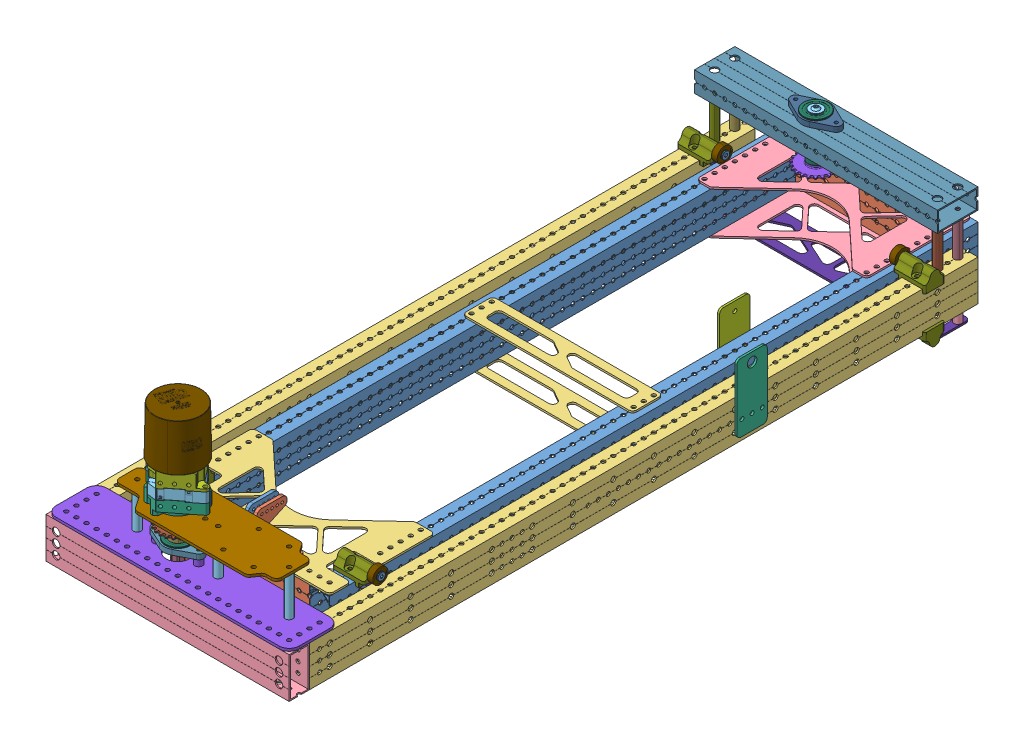
SolidWorks assembly Elevator Assembly 3.0, configuration Default. Lengths in mm.
Overall size (311.03 238.34 907.36).
103 component instances, 46 part files, 163 mates.
Components (placement in the parent):
- 32inTubeStock-1: 32inTubeStock [Default] at (147.012 423.1257 1446.8134) size (25.4 50.8 812.8)
- 32inTubeStock-2: 32inTubeStock [Default] at (-56.188 423.1257 1446.8134) size (25.4 50.8 812.8)
- 7inRevTube-1: 7inRevTube [Default] at (1137.612 423.1257 1065.8134) x (0 0 -1) z (1 0 0) size (25.4 50.8 177.8)
- 7inRevTube-2: 7inRevTube [Default] at (1137.612 423.1257 278.4134) x (0 0 -1) z (1 0 0) size (25.4 50.8 177.8)
- WCP-EX-0018-005(2)^Assem1-1: WCP-EX-0018-005(2)^Assem1 [Default] at (185.112 423.1257 519.7134) x (0 0 1) z (-1 0 0) size (838.2 50.8 25.4)
- WCP-EX-0018-001(2)^Assem1-1: WCP-EX-0018-001(2)^Assem1 [Default] at (45.412 423.1257 1154.7134) size (304.8 50.8 25.4)
- WCP-EX-0018-005(2)^Assem1-2: WCP-EX-0018-005(2)^Assem1 [Default] at (-94.288 423.1257 519.7134) x (0 0 1) z (-1 0 0) size (838.2 50.8 25.4)
- REV-21-2102-4-1-cartridge-1: REV-21-2102-4-1-cartridge [Default] at (20.0926 531.0257 1129.1434) x (0.78617 0 -0.61801) z (0 -1 0) size (61.91 50.8 16.85)
- REV-21-2104-hex-socket-output-1: REV-21-2104-hex-socket-output [Default] at (20.0961 515.2007 1129.1406) x (0 -1 0) z (-0.78617 0 0.61801) size (23.2 50.8 61.92)
- REV-21-2106-universal-input-1: REV-21-2106-universal-input [Default] at (20.0926 546.8507 1129.1434) x (0.78617 0 -0.61801) z (0 -1 0) size (61.91 50.8 19.05)
- Copy (3) of Copy of WCP-0308 Rev1^Elevator Assembly 3.0-3: Copy (3) of Copy of WCP-0308 Rev1^Elevator Assembly 3.0 [Default] at (45.4854 454.8757 1128.4014) x (0 1 0) z (-0.838797 0 -0.544444) size (8.64 9.5 9.6) (virtual)
- Motor_Mounting_Plate-1: Motor_Mounting_Plate [Default] at (-30.7773 505.6757 1129.3134) x (1 0 0) z (0 0 -1) size (209.55 3.17 69.85)
- Copy of Copy of WCP-0800_500_hex_collar_high_strength^Elevator Assembly 3.0-1: Copy of Copy of WCP-0800_500_hex_collar_high_strength^Elevator Assembly 3.0 [Default] at (20.0961 492.0867 1129.1406) x (0.837169 0 0.546944) z (0 1 0) size (28.56 28.57 9.53) (virtual)
- Copy of Copy of WCP-0560 Rev1^Elevator Assembly 3.0-1: Copy of Copy of WCP-0560 Rev1^Elevator Assembly 3.0 [Default] at (20.0961 482.5617 1129.1406) x (0.312597 0 0.949886) z (0 -1 0) size (47.96 47.68 9.53) (virtual)
- Copy of Copy of WCP-0789_250L_500_hex^Elevator Assembly 3.0-1: Copy of Copy of WCP-0789_250L_500_hex^Elevator Assembly 3.0 [Default] at (20.0961 471.4492 1129.1406) x (-0.74566 0 -0.666327) z (0 1 0) size (19.5 19.5 6.35) (virtual)
- 1_2ThunderHex-1: 1_2ThunderHex [Default] at (20.0961 872.3882 1129.1406) x (0.204226 0 -0.978924) z (0 1 0) size (13.74 12.75 101.6)
- Copy of Copy of WCP-0476 Rev1^Elevator Assembly 3.0-1: Copy of Copy of WCP-0476 Rev1^Elevator Assembly 3.0 [Default] at (20.0961 463.5117 1129.1406) x (-0.999576 0 0.029102) z (0 -1 0) size (63.5 34.92 6.35) (virtual)
- WCP-0785_0_500_flanged_thunderhex_bearing.step-3: WCP-0785_0_500_flanged_thunderhex_bearing.step [Default] at (20.0961 464.3055 1129.1406) x (0.837169 0 0.546944) z (0 1 0) size (31.12 31.12 7.94)
- Copy (3) of Copy of WCP-0308 Rev1^Elevator Assembly 3.0-4: Copy (3) of Copy of WCP-0308 Rev1^Elevator Assembly 3.0 [Default] at (-5.2931 454.8757 1129.8798) x (0 1 0) z (0.450792 0 -0.892629) size (8.64 9.5 9.6) (virtual)
- Copy of WCP-0323 - Elevator Clamping Block-1-1: Copy of WCP-0323 - Elevator Clamping Block-1 [Default] at (159.7755 448.5257 1034.0634) x (0 -1 0) z (1 0 0) size (29.22 25.41 49.35)
  - WCP-0323-001 Rev2^Copy of WCP-0323 - Elevator Clamping Block-1-1: WCP-0323-001 Rev2^Copy of WCP-0323 - Elevator Clamping Block-1 [Default] at origin size (20.38 25.41 40.49) (virtual)
  - WCP-0498 Rev1^Copy of WCP-0323 - Elevator Clamping Block-1-1: WCP-0498 Rev1^Copy of WCP-0323 - Elevator Clamping Block-1 [Default] at (2.254 0 6.7) x (0 0.307359 0.951594) z (-1 0 0) size (12 12 4) (virtual)
  - WCP-0212_0_250_radial_bearing^Copy of WCP-0323 - Elevator Clamping Block-1-1: WCP-0212_0_250_radial_bearing^Copy of WCP-0323 - Elevator Clamping Block-1 [Default] at (-9.525 0 15.4781) size (19.05 19.05 7.14) (virtual)
  - WCP-0473 Rev1^Copy of WCP-0323 - Elevator Clamping Block-1-1: WCP-0473 Rev1^Copy of WCP-0323 - Elevator Clamping Block-1 [Default] at (-9.525 0 10.4394) x (-0.082744 -0.996571 0) z (-0.996571 0.082744 0) size (9.53 20.65 9.53) (virtual)
  - #8-32 x .25L BHCS^Copy of WCP-0323 - Elevator Clamping Block-1-1: #8-32 x .25L BHCS^Copy of WCP-0323 - Elevator Clamping Block-1 [Default] at (6.7178 0 6.7) x (0 -0.337236 -0.94142) z (1 0 0) size (10.28 8 12.02) (virtual)
- Inside_Bottom_Plate-1: Inside_Bottom_Plate [Default] at (-738.7858 448.5257 1008.0258) x (0 0 1) z (0 1 0) size (132.08 228.6 2.29)
- Copy of WCP-0323 - Elevator Clamping Block-1-2: Copy of WCP-0323 - Elevator Clamping Block-1 [Default] at (172.3485 448.5257 360.9634) x (0 -1 0) z (-1 0 0) size (29.22 25.41 49.35)
  - WCP-0323-001 Rev2^Copy of WCP-0323 - Elevator Clamping Block-1-1: WCP-0323-001 Rev2^Copy of WCP-0323 - Elevator Clamping Block-1 [Default] at origin size (20.38 25.41 40.49) (virtual)
  - WCP-0498 Rev1^Copy of WCP-0323 - Elevator Clamping Block-1-1: WCP-0498 Rev1^Copy of WCP-0323 - Elevator Clamping Block-1 [Default] at (2.254 0 6.7) x (0 0.307359 0.951594) z (-1 0 0) size (12 12 4) (virtual)
  - WCP-0212_0_250_radial_bearing^Copy of WCP-0323 - Elevator Clamping Block-1-1: WCP-0212_0_250_radial_bearing^Copy of WCP-0323 - Elevator Clamping Block-1 [Default] at (-9.525 0 15.4781) size (19.05 19.05 7.14) (virtual)
  - WCP-0473 Rev1^Copy of WCP-0323 - Elevator Clamping Block-1-1: WCP-0473 Rev1^Copy of WCP-0323 - Elevator Clamping Block-1 [Default] at (-9.525 0 10.4394) x (-0.082744 -0.996571 0) z (-0.996571 0.082744 0) size (9.53 20.65 9.53) (virtual)
  - #8-32 x .25L BHCS^Copy of WCP-0323 - Elevator Clamping Block-1-1: #8-32 x .25L BHCS^Copy of WCP-0323 - Elevator Clamping Block-1 [Default] at (6.7178 0 6.7) x (0 -0.337236 -0.94142) z (1 0 0) size (10.28 8 12.02) (virtual)
- Inside_Top_Plate-1: Inside_Top_Plate [Default] at (712.3991 448.5257 509.6002) x (0 0 -1) z (0 1 0) size (132.08 213.36 2.29)
- Copy of Copy of WCP-0571 Rev1^Elevator Assembly 3.0-1: Copy of Copy of WCP-0571 Rev1^Elevator Assembly 3.0 [Default] at (20.012 535.6604 329.2134) x (-0.49457 0 -0.869138) z (0 1 0) size (15.88 15.88 15.71) (virtual)
- Copy (2) of Copy of WCP-0571 Rev1^Elevator Assembly 3.0-2: Copy (2) of Copy of WCP-0571 Rev1^Elevator Assembly 3.0 [Default] at (20.012 466.166 329.2134) x (-0.946289 0 0.323321) z (0 -1 0) size (15.88 15.88 15.71) (virtual)
- Copy of Copy of WCP-0599 Rev1^Elevator Assembly 3.0-1: Copy of Copy of WCP-0599 Rev1^Elevator Assembly 3.0 [Default] at (20.012 500.9132 329.2134) x (0 -1 0) z (-0.783433 0 0.621476) size (63.5 12.67 13.72) (virtual)
- Copy of Copy (2) of WCP-0560 Rev1^Elevator Assembly 3.0-1: Copy of Copy (2) of WCP-0560 Rev1^Elevator Assembly 3.0 [Default] at (20.012 473.9257 329.2134) x (0.367735 0 -0.929931) z (0 -1 0) size (47.96 47.68 9.53) (virtual)
- WCP-0785_0_500_flanged_thunderhex_bearing.step-4: WCP-0785_0_500_flanged_thunderhex_bearing.step [Default] at (20.012 495.357 329.2134) x (-0.189996 0 -0.981785) z (0 -1 0) size (31.12 31.12 7.94)
- Copy (2) of Copy of WCP-0476 Rev1^Elevator Assembly 3.0-2: Copy (2) of Copy of WCP-0476 Rev1^Elevator Assembly 3.0 [Default] at (20.012 496.1507 329.2134) x (1 0 0) z (0 1 0) size (63.5 34.92 6.35) (virtual)
- WCP-0785_0_500_flanged_thunderhex_bearing.step-5: WCP-0785_0_500_flanged_thunderhex_bearing.step [Default] at (20.012 528.6945 329.2134) x (0.679938 0 -0.73327) z (0 1 0) size (31.12 31.12 7.94)
- Copy (3) of Copy of WCP-0476 Rev1^Elevator Assembly 3.0-3: Copy (3) of Copy of WCP-0476 Rev1^Elevator Assembly 3.0 [Default] at (20.012 527.9007 329.2134) x (1 0 0) z (0 -1 0) size (63.5 34.92 6.35) (virtual)
- Copy of Copy of WCP-0207 Rev1^Elevator Assembly 3.0-1: Copy of Copy of WCP-0207 Rev1^Elevator Assembly 3.0 [Default] at (185.112 473.9257 341.9134) x (0 -1 0) z (-0.448341 0 -0.893863) size (50.8 9.5 9.5) (virtual)
- Copy (2) of Copy of WCP-0207 Rev1^Elevator Assembly 3.0-2: Copy (2) of Copy of WCP-0207 Rev1^Elevator Assembly 3.0 [Default] at (-94.288 473.9257 316.5134) x (0 -1 0) z (-0.997465 0 0.071155) size (50.8 9.5 9.5) (virtual)
- Copy (3) of Copy of WCP-0207 Rev1^Elevator Assembly 3.0-3: Copy (3) of Copy of WCP-0207 Rev1^Elevator Assembly 3.0 [Default] at (185.112 473.9257 316.5134) x (0 -1 0) z (0.909972 0 0.414669) size (50.8 9.5 9.5) (virtual)
- WCP-EX-0018-002(2)^Elevator Assembly Updated 2.0-2: WCP-EX-0018-002(2)^Elevator Assembly Updated 2.0 [Default] at (45.412 512.0257 329.2134) x (1 0 0) z (0 -1 0) size (304.8 50.8 25.4)
- WCP-0790_500L_500_hex.step-1: WCP-0790_500L_500_hex.step [Default] at (20.012 485.0382 329.2134) x (0.992611 0 -0.121342) z (0 -1 0) size (19.5 19.5 12.7)
- Copy (4) of Copy of WCP-0207 Rev1^Elevator Assembly 3.0-4: Copy (4) of Copy of WCP-0207 Rev1^Elevator Assembly 3.0 [Default] at (-94.288 473.9257 341.9134) x (0 -1 0) z (0.710119 0 0.704082) size (50.8 9.5 9.5) (virtual)
- Outside_Top_Plate-1: Outside_Top_Plate [Default] at (185.112 378.6757 316.5134) x (0 0 1) z (0 -1 0) size (45.72 289.24 2.29)
- Part4^Elevator Assembly 3.0-1: Part4^Elevator Assembly 3.0 [Default] at origin (virtual)
- Neo1.1_REV-21-1650-V1.1-1: Neo1.1_REV-21-1650-V1.1 [Default] at (20.0926 556.3757 1129.1434) x (0.451737 0 0.892151) z (0 -1 0) size (68.13 68.01 93.35)
- Copy of WCP-0323 - Elevator Clamping Block-1-9: Copy of WCP-0323 - Elevator Clamping Block-1 [Default] at (-68.9515 448.5257 1034.0634) x (0 -1 0) z (-1 0 0) size (29.22 25.41 49.35)
  - WCP-0323-001 Rev2^Copy of WCP-0323 - Elevator Clamping Block-1-1: WCP-0323-001 Rev2^Copy of WCP-0323 - Elevator Clamping Block-1 [Default] at origin size (20.38 25.41 40.49) (virtual)
  - WCP-0498 Rev1^Copy of WCP-0323 - Elevator Clamping Block-1-1: WCP-0498 Rev1^Copy of WCP-0323 - Elevator Clamping Block-1 [Default] at (2.254 0 6.7) x (0 0.307359 0.951594) z (-1 0 0) size (12 12 4) (virtual)
  - WCP-0212_0_250_radial_bearing^Copy of WCP-0323 - Elevator Clamping Block-1-1: WCP-0212_0_250_radial_bearing^Copy of WCP-0323 - Elevator Clamping Block-1 [Default] at (-9.525 0 15.4781) size (19.05 19.05 7.14) (virtual)
  - WCP-0473 Rev1^Copy of WCP-0323 - Elevator Clamping Block-1-1: WCP-0473 Rev1^Copy of WCP-0323 - Elevator Clamping Block-1 [Default] at (-9.525 0 10.4394) x (-0.082744 -0.996571 0) z (-0.996571 0.082744 0) size (9.53 20.65 9.53) (virtual)
  - #8-32 x .25L BHCS^Copy of WCP-0323 - Elevator Clamping Block-1-1: #8-32 x .25L BHCS^Copy of WCP-0323 - Elevator Clamping Block-1 [Default] at (6.7178 0 6.7) x (0 -0.337236 -0.94142) z (1 0 0) size (10.28 8 12.02) (virtual)
- Copy of WCP-0323 - Elevator Clamping Block-1-10: Copy of WCP-0323 - Elevator Clamping Block-1 [Default] at (-81.5245 448.5257 360.9634) x (0 -1 0) z (1 0 0) size (29.22 25.41 49.35)
  - WCP-0323-001 Rev2^Copy of WCP-0323 - Elevator Clamping Block-1-1: WCP-0323-001 Rev2^Copy of WCP-0323 - Elevator Clamping Block-1 [Default] at origin size (20.38 25.41 40.49) (virtual)
  - WCP-0498 Rev1^Copy of WCP-0323 - Elevator Clamping Block-1-1: WCP-0498 Rev1^Copy of WCP-0323 - Elevator Clamping Block-1 [Default] at (2.254 0 6.7) x (0 0.307359 0.951594) z (-1 0 0) size (12 12 4) (virtual)
  - WCP-0212_0_250_radial_bearing^Copy of WCP-0323 - Elevator Clamping Block-1-1: WCP-0212_0_250_radial_bearing^Copy of WCP-0323 - Elevator Clamping Block-1 [Default] at (-9.525 0 15.4781) size (19.05 19.05 7.14) (virtual)
  - WCP-0473 Rev1^Copy of WCP-0323 - Elevator Clamping Block-1-1: WCP-0473 Rev1^Copy of WCP-0323 - Elevator Clamping Block-1 [Default] at (-9.525 0 10.4394) x (-0.082744 -0.996571 0) z (-0.996571 0.082744 0) size (9.53 20.65 9.53) (virtual)
  - #8-32 x .25L BHCS^Copy of WCP-0323 - Elevator Clamping Block-1-1: #8-32 x .25L BHCS^Copy of WCP-0323 - Elevator Clamping Block-1 [Default] at (6.7178 0 6.7) x (0 -0.337236 -0.94142) z (1 0 0) size (10.28 8 12.02) (virtual)
- Copy of WCP-0323 - Elevator Clamping Block-1-15: Copy of WCP-0323 - Elevator Clamping Block-1 [Default] at (159.7755 397.7257 1034.0634) x (0 1 0) z (1 0 0) size (29.22 25.41 49.35)
  - WCP-0323-001 Rev2^Copy of WCP-0323 - Elevator Clamping Block-1-1: WCP-0323-001 Rev2^Copy of WCP-0323 - Elevator Clamping Block-1 [Default] at origin size (20.38 25.41 40.49) (virtual)
  - WCP-0498 Rev1^Copy of WCP-0323 - Elevator Clamping Block-1-1: WCP-0498 Rev1^Copy of WCP-0323 - Elevator Clamping Block-1 [Default] at (2.254 0 6.7) x (0 0.307359 0.951594) z (-1 0 0) size (12 12 4) (virtual)
  - WCP-0212_0_250_radial_bearing^Copy of WCP-0323 - Elevator Clamping Block-1-1: WCP-0212_0_250_radial_bearing^Copy of WCP-0323 - Elevator Clamping Block-1 [Default] at (-9.525 0 15.4781) size (19.05 19.05 7.14) (virtual)
  - WCP-0473 Rev1^Copy of WCP-0323 - Elevator Clamping Block-1-1: WCP-0473 Rev1^Copy of WCP-0323 - Elevator Clamping Block-1 [Default] at (-9.525 0 10.4394) x (-0.082744 -0.996571 0) z (-0.996571 0.082744 0) size (9.53 20.65 9.53) (virtual)
  - #8-32 x .25L BHCS^Copy of WCP-0323 - Elevator Clamping Block-1-1: #8-32 x .25L BHCS^Copy of WCP-0323 - Elevator Clamping Block-1 [Default] at (6.7178 0 6.7) x (0 -0.337236 -0.94142) z (1 0 0) size (10.28 8 12.02) (virtual)
- Copy of WCP-0323 - Elevator Clamping Block-1-16: Copy of WCP-0323 - Elevator Clamping Block-1 [Default] at (172.3485 397.7257 360.9634) x (0 1 0) z (-1 0 0) size (29.22 25.41 49.35)
  - WCP-0323-001 Rev2^Copy of WCP-0323 - Elevator Clamping Block-1-1: WCP-0323-001 Rev2^Copy of WCP-0323 - Elevator Clamping Block-1 [Default] at origin size (20.38 25.41 40.49) (virtual)
  - WCP-0498 Rev1^Copy of WCP-0323 - Elevator Clamping Block-1-1: WCP-0498 Rev1^Copy of WCP-0323 - Elevator Clamping Block-1 [Default] at (2.254 0 6.7) x (0 0.307359 0.951594) z (-1 0 0) size (12 12 4) (virtual)
  - WCP-0212_0_250_radial_bearing^Copy of WCP-0323 - Elevator Clamping Block-1-1: WCP-0212_0_250_radial_bearing^Copy of WCP-0323 - Elevator Clamping Block-1 [Default] at (-9.525 0 15.4781) size (19.05 19.05 7.14) (virtual)
  - WCP-0473 Rev1^Copy of WCP-0323 - Elevator Clamping Block-1-1: WCP-0473 Rev1^Copy of WCP-0323 - Elevator Clamping Block-1 [Default] at (-9.525 0 10.4394) x (-0.082744 -0.996571 0) z (-0.996571 0.082744 0) size (9.53 20.65 9.53) (virtual)
  - #8-32 x .25L BHCS^Copy of WCP-0323 - Elevator Clamping Block-1-1: #8-32 x .25L BHCS^Copy of WCP-0323 - Elevator Clamping Block-1 [Default] at (6.7178 0 6.7) x (0 -0.337236 -0.94142) z (1 0 0) size (10.28 8 12.02) (virtual)
- Copy of WCP-0323 - Elevator Clamping Block-1-17: Copy of WCP-0323 - Elevator Clamping Block-1 [Default] at (-68.9515 397.7257 1034.0634) x (0 1 0) z (-1 0 0) size (29.22 25.41 49.35)
  - WCP-0323-001 Rev2^Copy of WCP-0323 - Elevator Clamping Block-1-1: WCP-0323-001 Rev2^Copy of WCP-0323 - Elevator Clamping Block-1 [Default] at origin size (20.38 25.41 40.49) (virtual)
  - WCP-0498 Rev1^Copy of WCP-0323 - Elevator Clamping Block-1-1: WCP-0498 Rev1^Copy of WCP-0323 - Elevator Clamping Block-1 [Default] at (2.254 0 6.7) x (0 0.307359 0.951594) z (-1 0 0) size (12 12 4) (virtual)
  - WCP-0212_0_250_radial_bearing^Copy of WCP-0323 - Elevator Clamping Block-1-1: WCP-0212_0_250_radial_bearing^Copy of WCP-0323 - Elevator Clamping Block-1 [Default] at (-9.525 0 15.4781) size (19.05 19.05 7.14) (virtual)
  - WCP-0473 Rev1^Copy of WCP-0323 - Elevator Clamping Block-1-1: WCP-0473 Rev1^Copy of WCP-0323 - Elevator Clamping Block-1 [Default] at (-9.525 0 10.4394) x (-0.082744 -0.996571 0) z (-0.996571 0.082744 0) size (9.53 20.65 9.53) (virtual)
  - #8-32 x .25L BHCS^Copy of WCP-0323 - Elevator Clamping Block-1-1: #8-32 x .25L BHCS^Copy of WCP-0323 - Elevator Clamping Block-1 [Default] at (6.7178 0 6.7) x (0 -0.337236 -0.94142) z (1 0 0) size (10.28 8 12.02) (virtual)
- Copy of WCP-0323 - Elevator Clamping Block-1-18: Copy of WCP-0323 - Elevator Clamping Block-1 [Default] at (-81.5245 397.7257 360.9634) x (0 1 0) z (1 0 0) size (29.22 25.41 49.35)
  - WCP-0323-001 Rev2^Copy of WCP-0323 - Elevator Clamping Block-1-1: WCP-0323-001 Rev2^Copy of WCP-0323 - Elevator Clamping Block-1 [Default] at origin size (20.38 25.41 40.49) (virtual)
  - WCP-0498 Rev1^Copy of WCP-0323 - Elevator Clamping Block-1-1: WCP-0498 Rev1^Copy of WCP-0323 - Elevator Clamping Block-1 [Default] at (2.254 0 6.7) x (0 0.307359 0.951594) z (-1 0 0) size (12 12 4) (virtual)
  - WCP-0212_0_250_radial_bearing^Copy of WCP-0323 - Elevator Clamping Block-1-1: WCP-0212_0_250_radial_bearing^Copy of WCP-0323 - Elevator Clamping Block-1 [Default] at (-9.525 0 15.4781) size (19.05 19.05 7.14) (virtual)
  - WCP-0473 Rev1^Copy of WCP-0323 - Elevator Clamping Block-1-1: WCP-0473 Rev1^Copy of WCP-0323 - Elevator Clamping Block-1 [Default] at (-9.525 0 10.4394) x (-0.082744 -0.996571 0) z (-0.996571 0.082744 0) size (9.53 20.65 9.53) (virtual)
  - #8-32 x .25L BHCS^Copy of WCP-0323 - Elevator Clamping Block-1-1: #8-32 x .25L BHCS^Copy of WCP-0323 - Elevator Clamping Block-1 [Default] at (6.7178 0 6.7) x (0 -0.337236 -0.94142) z (1 0 0) size (10.28 8 12.02) (virtual)
- Inside_Bottom_Plate-3: Inside_Bottom_Plate [Default] at (-738.7858 395.4397 1008.0258) x (0 0 1) z (0 1 0) size (132.08 228.6 2.29)
- WCP-0583-025 Rev1_DefaultSM-FLAT-PATTERN.step-1: WCP-0583-025 Rev1_DefaultSM-FLAT-PATTERN.step [Default] at (23.187 454.8117 1065.8134) x (1 0 0) z (0 1 0) size (44.45 50.8 31.75)
- WCP-0583-026 Rev1.step-1: WCP-0583-026 Rev1.step [Default] at (77.162 454.8117 1065.8134) x (1 0 0) z (0 1 0) size (50.8 50.8 31.75)
- Inside_Middle_Plate-1: Inside_Middle_Plate [Default] at (-56.188 448.5257 1446.8134) x (1 0 0) z (0 1 0) size (213.36 38.1 2.29)
- Inside_Middle_Plate-2: Inside_Middle_Plate [Default] at (-56.188 395.4397 1446.8134) x (1 0 0) z (0 1 0) size (213.36 38.1 2.29)
- 0_750_L_10_thru_WCP-0217-1: 0_750_L_10_thru_WCP-0217 [Default] at (-94.288 388.2007 341.9134) x (0 1 0) z (-0.160818 0 -0.986984) size (19.05 9.5 9.5)
- 0_750_L_10_thru_WCP-0217-2: 0_750_L_10_thru_WCP-0217 [Default] at (-94.288 388.2007 316.5134) x (0 1 0) z (-0.962052 0 -0.272865) size (19.05 9.5 9.5)
- 0_750_L_10_thru_WCP-0217-3: 0_750_L_10_thru_WCP-0217 [Default] at (185.112 388.2007 341.9134) x (0 1 0) z (0.167347 0 0.985898) size (19.05 9.5 9.5)
- 0_750_L_10_thru_WCP-0217-5: 0_750_L_10_thru_WCP-0217 [Default] at (185.112 388.2007 316.5134) x (0 1 0) z (0.00547 0 -0.999985) size (19.05 9.5 9.5)
- Inside_Top_Plate-2: Inside_Top_Plate [Default] at (712.3991 395.4397 509.6002) x (0 0 -1) z (0 1 0) size (132.08 213.36 2.29)
- 2_000_L_10_thru_WCP-0207-1: 2_000_L_10_thru_WCP-0207 [Default] at (70.8227 477.1007 1129.3134) x (0 -1 0) z (-0.252114 0 0.967698) size (50.8 9.5 9.5)
- 2_000_L_10_thru_WCP-0207-2: 2_000_L_10_thru_WCP-0207 [Default] at (-30.7773 477.1007 1129.3134) x (0 -1 0) z (0.923494 0 0.383613) size (50.8 9.5 9.5)
- 2_000_L_10_thru_WCP-0207-3: 2_000_L_10_thru_WCP-0207 [Default] at (159.7227 477.1007 1129.3134) x (0 -1 0) z (-0.72729 0 0.68633) size (50.8 9.5 9.5)
- Part5^Elevator Assembly 3.0-1: Part5^Elevator Assembly 3.0 [Default] at (197.812 423.1257 221.2634) x (0 0 -1) z (1 0 0) size (38.1 85.66 2.54) (virtual)
- Copy of Part5^Elevator Assembly 3.0-1: Copy of Part5^Elevator Assembly 3.0 [Default] at (131.772 423.1257 176.8134) x (0 0 -1) z (1 0 0) size (38.1 85.66 2.54) (virtual)
- New_Motor_Mounting_Plate-1: New_Motor_Mounting_Plate [Default] at (197.812 448.5257 1103.9134) x (-1 0 0) z (0 0 -1) size (304.8 3.17 63.5)
- 0_125_L_500_hex_spacer_217-2758-2: 0_125_L_500_hex_spacer_217-2758 [Default] at (20.0961 476.2117 1129.1406) x (0.666327 0 -0.74566) z (0 -1 0) size (19.05 19.05 3.17)
Mates (geometry in assembly coordinates):
- Coincident1: coincident aligned: plane of 32inTubeStock-1 through (147.012 423.1257 1078.5134) normal (0 0 1); plane of 32inTubeStock-2 through (-56.188 423.1257 1078.5134) normal (0 0 1)
- Coincident2: coincident aligned: plane of 32inTubeStock-1 through (159.712 448.5257 265.7134) normal (0 1 0); plane of 32inTubeStock-2 through (-43.488 448.5257 265.7134) normal (0 1 0)
- Coincident3: coincident aligned: plane of 32inTubeStock-2 through (-43.488 448.5257 265.7134) normal (0 1 0); plane of 7inRevTube-1 through (-43.488 448.5257 1053.1134) normal (0 1 0)
- Coincident4: coincident anti-aligned: plane of 32inTubeStock-1 through (134.312 397.7257 265.7134) normal (-1 0 0); plane of 7inRevTube-1 through (134.312 423.1257 1065.8134) normal (1 0 0)
- Coincident5: coincident aligned: plane of 32inTubeStock-1 through (147.012 423.1257 1078.5134) normal (0 0 1); plane of 7inRevTube-1 through (-43.488 397.7257 1078.5134) normal (0 0 1)
- Coincident6: coincident anti-aligned: plane of 32inTubeStock-2 through (-43.488 397.7257 265.7134) normal (1 0 0); plane of 7inRevTube-1 through (-43.488 423.1257 1065.8134) normal (-1 0 0)
- Coincident7: coincident aligned: plane of 7inRevTube-1 through (-43.488 448.5257 1053.1134) normal (0 1 0); plane of 7inRevTube-2 through (-43.488 448.5257 265.7134) normal (0 1 0)
- Coincident8: coincident anti-aligned: plane of 32inTubeStock-2 through (-43.488 397.7257 265.7134) normal (1 0 0); plane of 7inRevTube-2 through (-43.488 423.1257 278.4134) normal (-1 0 0)
- Coincident9: coincident aligned: plane of 32inTubeStock-2 through (-56.188 423.1257 265.7134) normal (0 0 -1); plane of 7inRevTube-2 through (-43.488 397.7257 265.7134) normal (0 0 -1)
- Parallel1: parallel anti-aligned: plane of 32inTubeStock-1 through (159.712 397.7257 265.7134) normal (1 0 0); plane of WCP-EX-0018-005(2)^Assem1-1 through (172.412 397.7257 1116.6134) normal (-1 0 0)
- Coincident12: coincident aligned: plane of 7inRevTube-1 through (-43.488 448.5257 1053.1134) normal (0 1 0); plane of WCP-EX-0018-005(2)^Assem1-1 through (172.412 448.5257 1116.6134) normal (0 1 0)
- Coincident13: coincident anti-aligned: plane of WCP-EX-0018-005(2)^Assem1-1 through (185.112 423.1257 1142.0134) normal (0 0 1); plane of WCP-EX-0018-001(2)^Assem1-1 through (235.912 397.7257 1142.0134) normal (0 0 -1)
- Coincident14: coincident aligned: plane of WCP-EX-0018-005(2)^Assem1-1 through (172.412 448.5257 1116.6134) normal (0 1 0); plane of WCP-EX-0018-001(2)^Assem1-1 through (235.912 448.5257 1167.4134) normal (0 1 0)
- Coincident15: coincident aligned: plane of WCP-EX-0018-005(2)^Assem1-1 through (197.812 397.7257 1116.6134) normal (1 0 0); plane of WCP-EX-0018-001(2)^Assem1-1 through (197.812 397.7257 1167.4134) normal (1 0 0)
- Coincident16: coincident aligned: plane of WCP-EX-0018-001(2)^Assem1-1 through (235.912 448.5257 1167.4134) normal (0 1 0); plane of WCP-EX-0018-005(2)^Assem1-2 through (-106.988 448.5257 1116.6134) normal (0 1 0)
- Coincident20: coincident aligned: plane of 7inRevTube-1 through (-43.488 448.5257 1053.1134) normal (0 1 0); plane of WCP-EX-0018-001(2)^Assem1-1 through (235.912 448.5257 1167.4134) normal (0 1 0)
- Concentric4: concentric anti-aligned: cylinder of Copy of Copy of WCP-0800_500_hex_collar_high_strength^Elevator Assembly 3.0-1 through (20.0961 496.8492 1129.1406) axis (0 -1 0) radius 14.2875; cylinder of WCP-0785_0_500_flanged_thunderhex_bearing.step-3 through (20.0961 517.5544 1129.1406) axis (0 1 0) radius 6.875
- Concentric5: concentric aligned: cylinder of REV-21-2104-hex-socket-output-1 through (20.0961 524.7257 1129.1406) axis (0 1 0) radius 16; cylinder of 1_2ThunderHex-1 through (20.0961 415.1882 1129.1406) axis (0 1 0) radius 2.55
- Concentric9: concentric anti-aligned: cylinder of Copy of Copy of WCP-0560 Rev1^Elevator Assembly 3.0-1 through (20.0961 477.7992 1129.1406) axis (0 1 0) radius 9.525; cylinder of Copy of Copy of WCP-0789_250L_500_hex^Elevator Assembly 3.0-1 through (20.0961 474.6242 1129.1406) axis (0 -1 0) radius 9.75
- Concentric10: concentric aligned: cylinder of REV-21-2104-hex-socket-output-1 through (-14.3689 524.7257 1128.9733) axis (0 1 0) radius 2.0193; cylinder of REV-21-2106-universal-input-1 through (-14.3689 537.3257 1128.9733) axis (0 1 0) radius 2.5
- Concentric11: concentric aligned: cylinder of Copy of Copy of WCP-0476 Rev1^Elevator Assembly 3.0-1 through (20.0961 460.3367 1129.1406) axis (0 1 0) radius 14.2875; cylinder of WCP-0785_0_500_flanged_thunderhex_bearing.step-3 through (20.0961 517.5544 1129.1406) axis (0 1 0) radius 14.2875
- Concentric12: concentric anti-aligned: cylinder of Copy of Copy of WCP-0789_250L_500_hex^Elevator Assembly 3.0-1 through (20.0961 474.6242 1129.1406) axis (0 -1 0) radius 9.75; cylinder of 1_2ThunderHex-1 through (20.0961 415.1882 1129.1406) axis (0 1 0) radius 2.55
- Concentric13: concentric aligned: cylinder of Copy (3) of Copy of WCP-0308 Rev1^Elevator Assembly 3.0-3 through (45.4854 458.0507 1128.4014) axis (0 -1 0) radius 4.7498; cylinder of Copy of Copy of WCP-0476 Rev1^Elevator Assembly 3.0-1 through (45.4854 460.3367 1128.4014) axis (0 -1 0) radius 2.0193
- Concentric16: concentric aligned: circle of Copy of Copy of WCP-0800_500_hex_collar_high_strength^Assem1-1; cylinder of 1_2ThunderHex-1 through (20.0961 415.1882 1129.1406) axis (0 1 0) radius 2.55
- Concentric17: concentric anti-aligned: cylinder of REV-21-2102-4-1-cartridge-1 through (-14.3689 524.6757 1128.9733) axis (0 -1 0) radius 2.5; cylinder of REV-21-2106-universal-input-1 through (-14.3689 537.3257 1128.9733) axis (0 1 0) radius 2.5
- Parallel3: parallel anti-aligned: plane of Copy of Copy of WCP-0789_250L_500_hex^Elevator Assembly 3.0-1 through (27.2003 474.6242 1126.8027) normal (-0.666327 0 0.74566); plane of 1_2ThunderHex-1 through (27.0889 1329.5882 1126.8394) normal (0.666327 0 -0.74566)
- Coincident21: coincident anti-aligned: plane of Copy of Copy of WCP-0476 Rev1^Elevator Assembly 3.0-1 through (20.0961 466.6867 1129.1406) normal (0 1 0); plane of WCP-0785_0_500_flanged_thunderhex_bearing.step-3 through (27.9106 466.6867 1117.1796) normal (0 -1 0)
- Coincident23: coincident anti-aligned: plane of Copy of Copy of WCP-0800_500_hex_collar_high_strength^Elevator Assembly 3.0-1 through (20.0961 487.3242 1129.1406) normal (0 -1 0); plane of Copy of Copy of WCP-0560 Rev1^Elevator Assembly 3.0-1 through (20.0961 487.3242 1129.1406) normal (0 1 0)
- Coincident24: coincident anti-aligned: plane of Copy of Copy of WCP-0560 Rev1^Elevator Assembly 3.0-1 through (14.6068 487.3242 1124.2353) normal (0.312597 0 0.949886); plane of 1_2ThunderHex-1 through (21.5996 1329.5882 1121.9341) normal (-0.312597 0 -0.949886)
- Coincident26: coincident anti-aligned: plane of Copy of Copy of WCP-0789_250L_500_hex^Elevator Assembly 3.0-1 through (20.0961 468.2742 1129.1406) normal (0 -1 0); plane of WCP-0785_0_500_flanged_thunderhex_bearing.step-3 through (25.3479 468.2742 1121.1021) normal (0 1 0)
- Coincident29: coincident aligned: plane of REV-21-2102-4-1-cartridge-1 through (24.3639 524.6757 1093.4772) normal (0.78617 0 -0.61801); plane of REV-21-2106-universal-input-1 through (40.0614 537.3257 1113.4459) normal (0.78617 0 -0.61801)
- Coincident30: coincident anti-aligned: plane of REV-21-2102-4-1-cartridge-1 through (20.0926 524.7257 1129.1434) normal (0 -1 0); plane of REV-21-2104-hex-socket-output-1 through (20.0961 524.7257 1129.1406) normal (0 1 0)
- Coincident32: coincident anti-aligned: plane of REV-21-2104-hex-socket-output-1 through (20.0961 516.7882 1129.1406) normal (0 -1 0); plane of 1_2ThunderHex-1 through (20.0961 516.7882 1129.1406) normal (0 1 0)
- Parallel4: parallel aligned: plane of REV-21-2104-hex-socket-output-1 through (60.1339 534.4172 1129.9753) normal (0.78617 0 -0.61801); plane of REV-21-2106-universal-input-1 through (40.0614 537.3257 1113.4459) normal (0.78617 0 -0.61801)
- Coincident35: coincident anti-aligned: plane of REV-21-2102-4-1-cartridge-1 through (20.0926 537.3257 1129.1434) normal (0 1 0); plane of REV-21-2106-universal-input-1 through (20.0926 537.3257 1129.1434) normal (0 -1 0)
- Coincident38: coincident anti-aligned: plane of Copy (3) of Copy of WCP-0308 Rev1^Elevator Assembly 3.0-3 through (45.4854 460.3367 1128.4014) normal (0 1 0); plane of Copy of Copy of WCP-0476 Rev1^Elevator Assembly 3.0-1 through (20.0961 460.3367 1129.1406) normal (0 -1 0)
- Concentric18: concentric aligned: cylinder of Copy of Copy of WCP-0476 Rev1^Elevator Assembly 3.0-1 through (-5.2931 460.3367 1129.8798) axis (0 -1 0) radius 2.0193; cylinder of Copy (3) of Copy of WCP-0308 Rev1^Elevator Assembly 3.0-4 through (-5.2931 458.0507 1129.8798) axis (0 -1 0) radius 2.4892
- Coincident39: coincident anti-aligned: plane of Copy of Copy of WCP-0476 Rev1^Elevator Assembly 3.0-1 through (20.0961 460.3367 1129.1406) normal (0 -1 0); plane of Copy (3) of Copy of WCP-0308 Rev1^Elevator Assembly 3.0-4 through (-5.2931 460.3367 1129.8798) normal (0 1 0)
- Angle4: planar angle = 0.481923 rad aligned: plane of Copy of Copy of WCP-0476 Rev1^Elevator Assembly 3.0-1 through (28.1897 460.3367 1144.6142) normal (0.463484 0 0.886105); plane of WCP-EX-0018-001(2)^Assem1-1 through (235.912 397.7257 1167.4134) normal (0 0 1)
- Coincident50: coincident anti-aligned: plane of WCP-EX-0018-001(2)^Assem1-1 through (235.912 397.7257 1142.0134) normal (0 0 -1); plane of WCP-EX-0018-005(2)^Assem1-2 through (-94.288 423.1257 1142.0134) normal (0 0 1)
